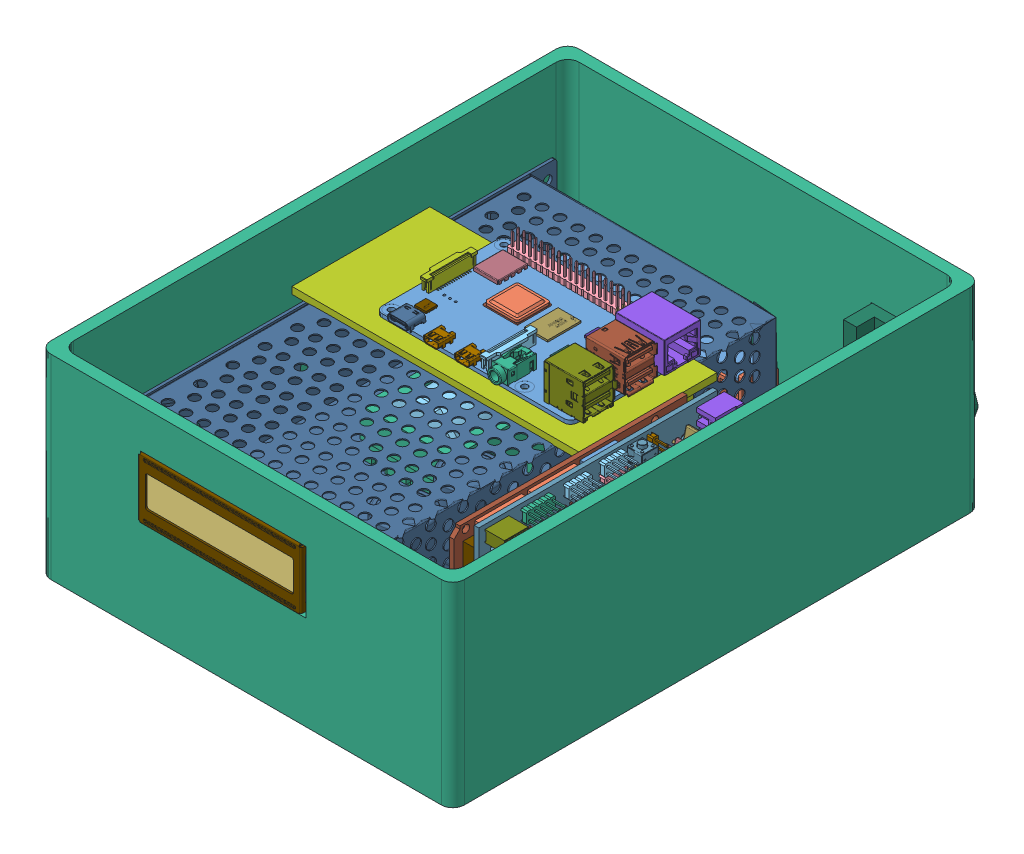
SolidWorks assembly Desktop_Arm_Assembly, configuration Default. Lengths in mm.
Overall size (180 85 238.3).
199 component instances, 97 part files, 19 mates.
Components (placement in the parent):
- Raspberry Pi 4 Model B-1: Raspberry Pi 4 Model B [Default] at (14.6782 37.9484 76.8197) size (88.99 19.9 58.4)
  - PCB, RPi4ModelB-1: PCB, RPi4ModelB [Default] at origin size (85 1.6 56)
  - Broadcom BCM2711B0 CPU, RPi4ModelB-1: Broadcom BCM2711B0 CPU, RPi4ModelB [Default] at (-13.25 0.8 -4.5) size (15 2.3 15)
  - 2.54 mm DUPONT MALE PIN HEADER, POE, 2X2, RPi4ModelB-1: 2.54 mm DUPONT MALE PIN HEADER, POE, 2X2, RPi4ModelB [Default] at (19 0.8 -18.5) size (5.08 11.3 5.08)
  - 2.54 mm DUPONT MALE PIN HEADER, IO, 2X20, RPi4ModelB-1: 2.54 mm DUPONT MALE PIN HEADER, IO, 2X20, RPi4ModelB [Default] at (-10 0.8 -24.5) size (50.8 11.3 5.08)
  - Camera Connector, RPi4ModelB-1: Camera Connector, RPi4ModelB [Default] at (4 0.8 16.5) x (0 0 -1) z (1 0 0) size (22.4 5.68 5.07)
  - Microphone Plug, RPi4ModelB-1: Microphone Plug, RPi4ModelB [Default] at (11.5 0.8 21.65) size (7.23 7.55 15)
  - Display Connector, RPi4ModelB-1: Display Connector, RPi4ModelB [Default] at (-38.5 0.8 0) x (0 0 1) z (-1 0 0) size (22.4 5.68 5.07)
  - Gigabit Ethernet Port, RPi4ModelB-1: Gigabit Ethernet Port, RPi4ModelB [Default] at (45.5 7.55 -17.75) x (0 0 -1) z (1 0 0) size (16.2 17.24 21.64)
  - Female Micro HDMI Connector, RPi4ModelB-2: Female Micro HDMI Connector, RPi4ModelB [Default] at (-3 0.8 27.3875) size (6.5 3.51 7.5)
  - Female Micro HDMI Connector, RPi4ModelB-3: Female Micro HDMI Connector, RPi4ModelB [Default] at (-16.5 0.8 27.3875) size (6.5 3.51 7.5)
  - Female USB Type C Connector, RPi4ModelB-1: Female USB Type C Connector, RPi4ModelB [Default] at (-31.3 0.8 26.5419) size (8.94 3.96 7.9)
  - 2X USB3.0 PORTS, RPi4ModelB-2: 2X USB3.0 PORTS, RPi4ModelB [Default] at (37.07 0.8 1) size (17.47 19.41 15.68)
  - 91D77 D9WHV 778K, 4 GB LPDDR4 SDRAM, RPi4ModelB-1: 91D77 D9WHV 778K, 4 GB LPDDR4 SDRAM, RPi4ModelB [Default] at (2.25 0.8 -4.5) size (10 0.8 14.5)
  - Cypress CYW43455 Wireless Module Cover, RPi4ModelB-1: Cypress CYW43455 Wireless Module Cover, RPi4ModelB [Default] at (-30.5 0.8 -14.5) size (11 1.6 13)
  - SD Card Slot, RPi4ModelB-1: SD Card Slot, RPi4ModelB [Default] at (-35.3 -0.8 0) x (0 0 -1) z (-1 0 0) size (11.95 1.45 11.4)
  - VIA VL805 PCIe USB 3.0 controller, RPi4ModelB-1: VIA VL805 PCIe USB 3.0 controller, RPi4ModelB [Default] at (17.5 0.8 4) size (8.8 0.8 8.8)
  - 2X USB2.0 PORTS, RPi4ModelB-1: 2X USB2.0 PORTS, RPi4ModelB [Default] at (37.065 0.65 19) size (17.87 19.16 15.33)
  - Broadcom BCM54213PE Gigabit Ethernet Transceiver, RPi4ModelB-1: Broadcom BCM54213PE Gigabit Ethernet Transceiver, RPi4ModelB [Default] at (16.5 0.8 -10) size (6.8 1 6.8)
  - MxL7704 Universal PMIC, RPi4ModelB-1: MxL7704 Universal PMIC, RPi4ModelB [Default] at (-32.5 0.8 16) size (5.4 0.8 5.4)
- PowerSupply_S-240-12.step-1: PowerSupply_S-240-12.step [Default] at (2.5782 -11.3016 98.3197) x (0 0 -1) z (0 1 0) size (202.29 118.05 58.32)
  - ScrewTerminalBlock_1x9.step-1: ScrewTerminalBlock_1x9.step [Default] at origin size (16 87.5 20.2)
    - SOLID007.step-1: SOLID007.step [Default] at origin size (14.65 87.4 2.8)
    - SOLID008.step-1: SOLID008.step [Default] at origin size (16 87.5 16.5)
    - SOLID009.step-1: SOLID009.step [Default] at origin size (9.8 7.4 11.5)
    - SOLID010.step-1: SOLID010.step [Default] at origin size (7.4 7.4 9.45)
    - SOLID011.step-1: SOLID011.step [Default] at origin size (9.8 7.4 11.5)
    - SOLID012.step-1: SOLID012.step [Default] at origin size (7.4 7.4 9.45)
    - SOLID013.step-1: SOLID013.step [Default] at origin size (9.8 7.4 11.5)
    - SOLID014.step-1: SOLID014.step [Default] at origin size (7.4 7.4 9.45)
    - SOLID015.step-1: SOLID015.step [Default] at origin size (9.8 7.4 11.5)
    - SOLID016.step-1: SOLID016.step [Default] at origin size (7.4 7.4 9.45)
    - SOLID017.step-1: SOLID017.step [Default] at origin size (9.8 7.4 11.5)
    - SOLID018.step-1: SOLID018.step [Default] at origin size (7.4 7.4 9.45)
    - SOLID019.step-1: SOLID019.step [Default] at origin size (9.8 7.4 11.5)
    - SOLID020.step-1: SOLID020.step [Default] at origin size (7.4 7.4 9.45)
    - SOLID021.step-1: SOLID021.step [Default] at origin size (9.8 7.4 11.5)
    - SOLID022.step-1: SOLID022.step [Default] at origin size (7.4 7.4 9.45)
    - SOLID023.step-1: SOLID023.step [Default] at origin size (9.8 7.4 11.5)
    - SOLID024.step-1: SOLID024.step [Default] at origin size (7.4 7.4 9.45)
    - SOLID025.step-1: SOLID025.step [Default] at origin size (9.8 7.4 11.5)
    - SOLID026.step-1: SOLID026.step [Default] at origin size (7.4 7.4 9.45)
  - Common_Mode_Choke.step-1: Common_Mode_Choke.step [Default] at origin size (18.5 21.5 27.15)
    - SOLID.step-1: SOLID.step [Default] at origin size (6 21.5 16.6)
    - SOLID001.step-1: SOLID001.step [Default] at origin size (18.5 16.8 21.5)
  - Trafo_TR01.step-1: Trafo_TR01.step [Default] at origin size (44 40 34.3)
    - SOLID002.step-1: SOLID002.step [Default] at origin size (31.6 28 24)
    - SOLID003.step-1: SOLID003.step [Default] at origin size (44 40 26.7)
  - Toroidal_Inductor-D30H24T030.step-1: Toroidal_Inductor-D30H24T030.step [Default] at origin size (36.95 37 26.57)
    - SOLID004.step-1: SOLID004.step [Default] at origin size (34.97 37 10)
    - SOLID005.step-1: SOLID005.step [Default] at origin size (34.97 37 10)
    - SOLID006.step-1: SOLID006.step [Default] at origin size (31.89 31.73 26.57)
  - eBom-FreeParts-1: eBom-FreeParts [Default] at origin size (202.29 118.05 58.32)
- hop dien.stp-1: hop dien.stp [Default] at (67.1652 328.6838 379.5226) x (0 -1 0) z (0 0 -1) size (61.76 43.8 111.7)
  - ARDUINO_MEGA.stp-1: ARDUINO_MEGA.stp [Default] at (319.6193 3.0542 265.0052) x (0 0 -1) z (-1 0 0) size (109.46 14.9 53.16)
    - ARDUINO_MEGA_BRD.stp-1: ARDUINO_MEGA_BRD.stp [Default] at (-33.9666 3.0673 -21.8675) x (1 0 0) z (0 1 0) size (101.46 53.16 2)
    - pin_header_aw140-eg-g02d.stp-1: pin_header_aw140-eg-g02d.stp [Default] at (16.2928 5.0673 -3.5536) x (-1 0 0) z (0 0 1) size (4.98 11.2 2.5)
    - pin_header_aw140-eg-g02d.stp-2: pin_header_aw140-eg-g02d.stp [Default] at (16.2928 5.0673 1.5635) x (-1 0 0) z (0 0 1) size (4.98 11.2 2.5)
    - pin_header_aw140-eg-g02d.stp-3: pin_header_aw140-eg-g02d.stp [Default] at (16.2928 5.0673 -1.1197) x (-1 0 0) z (0 0 1) size (4.98 11.2 2.5)
    - User Library-Arduino Mega_DC POWER JACK.stp-1: User Library-Arduino Mega_DC POWER JACK.stp [Default] at (-53.3977 5.0673 16.2059) x (0 0 1) z (-1 0 0) size (9.47 14.78 14.48)
    - User Library-Arduino Mega_USB SM host.stp-1: User Library-Arduino Mega_USB SM host.stp [Default] at (-48.1477 10.3173 -12.8661) x (0 0 1) z (-1 0 0) size (14.86 14.22 16.5)
    - User Library-Arduino Mega_Atmega1280 (WGL).stp-1: User Library-Arduino Mega_Atmega1280 (WGL).stp [Default] at (2.1792 5.0673 -1.4897) size (14 0.7 14)
    - User Library-Arduino Mega_tactile BUTTON.stp-1: User Library-Arduino Mega_tactile BUTTON.stp [Default] at (25.3856 5.0673 -0.9155) x (1 0 0) z (0 1 0) size (7.9 6.2 7.35)
    - User Library-Arduino Mega_SM LED.stp-1: User Library-Arduino Mega_SM LED.stp [Default] at (27.6088 5.0673 -9.939) size (2.8 1.12 1.4)
    - User Library-Arduino Mega_PIN HEADER FEMALE 2X18SLDPRT.stp-1: User Library-Arduino Mega_PIN HEADER FEMALE 2X18SLDPRT.stp [Default] at (47.9279 5.0673 19.0874) x (0 0 -1) z (1 0 0) size (45.04 8.3 5.08)
    - User Library-Arduino Mega_PIN HEADER FEMALE 6.stp-1: User Library-Arduino Mega_PIN HEADER FEMALE 6.stp [Default] at (-15.6783 5.0673 24.2251) size (15.24 8.3 2.54)
    - User Library-Arduino Mega_PIN HEADER FEMALE 8.stp-1: User Library-Arduino Mega_PIN HEADER FEMALE 8.stp [Default] at (2.1049 5.0673 24.3138) size (20.32 8.3 2.54)
    - User Library-Arduino Mega_PIN HEADER FEMALE 8.stp-2: User Library-Arduino Mega_PIN HEADER FEMALE 8.stp [Default] at (24.9983 5.0673 24.3138) size (20.32 8.3 2.54)
    - User Library-Arduino Mega_PIN HEADER FEMALE 8.stp-3: User Library-Arduino Mega_PIN HEADER FEMALE 8.stp [Default] at (19.9514 5.0673 -23.9148) size (20.32 8.3 2.54)
    - User Library-Arduino Mega_PIN HEADER FEMALE 8.stp-4: User Library-Arduino Mega_PIN HEADER FEMALE 8.stp [Default] at (-2.8895 5.0673 -23.9148) size (20.32 8.3 2.54)
    - User Library-Arduino Mega_PIN HEADER FEMALE 8.stp-5: User Library-Arduino Mega_PIN HEADER FEMALE 8.stp [Default] at (-24.6796 5.0673 -23.9148) size (20.32 8.3 2.54)
    - pin_header_aw254-dg-g06d.stp-1: pin_header_aw254-dg-g06d.stp [Default] at (-30.3155 5.0673 -19.3157) x (1 0 0) z (0 0 -1) size (7.62 11.5 5.08)
  - RAMPS1_4.stp-1: RAMPS1_4.stp [Default] at (314.7148 -10.7327 258.615) x (0 0 -1) z (-1 0 0) size (106.85 37.63 61.76)
    - User Library-CAPSMD6_3x3_9.stp-1: User Library-CAPSMD6_3x3_9.stp [Default] at (-23.4034 4.2803 -13.8521) x (0 0 -1) z (0 1 0) size (6.6 7 3.91)
      - User Library-CAPSMD6_3x3_9_CAP003.stp-1: User Library-CAPSMD6_3x3_9_CAP003.stp [Default] at origin size (0.65 2.6 0.32)
      - User Library-CAPSMD6_3x3_9_CAP.stp-1: User Library-CAPSMD6_3x3_9_CAP.stp [Default] at origin size (6.3 6.3 3.26)
      - User Library-CAPSMD6_3x3_9_CAP001.stp-1: User Library-CAPSMD6_3x3_9_CAP001.stp [Default] at origin size (6.6 6.6 0.64)
      - User Library-CAPSMD6_3x3_9_CAP002.stp-1: User Library-CAPSMD6_3x3_9_CAP002.stp [Default] at origin size (5.11 1.47 0.01)
      - User Library-CAPSMD6_3x3_9_CAP004.stp-1: User Library-CAPSMD6_3x3_9_CAP004.stp [Default] at origin size (0.65 2.6 0.32)
    - User Library-CAPSMD6_3x3_9.stp-2: User Library-CAPSMD6_3x3_9.stp [Default] at (-2.2688 4.2803 -13.8521) x (0 0 -1) z (0 1 0) size (6.6 7 3.91)
      - User Library-CAPSMD6_3x3_9_CAP003.stp-1: User Library-CAPSMD6_3x3_9_CAP003.stp [Default] at origin size (0.65 2.6 0.32)
      - User Library-CAPSMD6_3x3_9_CAP.stp-1: User Library-CAPSMD6_3x3_9_CAP.stp [Default] at origin size (6.3 6.3 3.26)
      - User Library-CAPSMD6_3x3_9_CAP001.stp-1: User Library-CAPSMD6_3x3_9_CAP001.stp [Default] at origin size (6.6 6.6 0.64)
      - User Library-CAPSMD6_3x3_9_CAP002.stp-1: User Library-CAPSMD6_3x3_9_CAP002.stp [Default] at origin size (5.11 1.47 0.01)
      - User Library-CAPSMD6_3x3_9_CAP004.stp-1: User Library-CAPSMD6_3x3_9_CAP004.stp [Default] at origin size (0.65 2.6 0.32)
    - User Library-CAPSMD6_3x3_9.stp-3: User Library-CAPSMD6_3x3_9.stp [Default] at (-2.8787 4.2803 9.2865) x (0 0 -1) z (0 1 0) size (6.6 7 3.91)
      - User Library-CAPSMD6_3x3_9_CAP003.stp-1: User Library-CAPSMD6_3x3_9_CAP003.stp [Default] at origin size (0.65 2.6 0.32)
      - User Library-CAPSMD6_3x3_9_CAP.stp-1: User Library-CAPSMD6_3x3_9_CAP.stp [Default] at origin size (6.3 6.3 3.26)
      - User Library-CAPSMD6_3x3_9_CAP001.stp-1: User Library-CAPSMD6_3x3_9_CAP001.stp [Default] at origin size (6.6 6.6 0.64)
      - User Library-CAPSMD6_3x3_9_CAP002.stp-1: User Library-CAPSMD6_3x3_9_CAP002.stp [Default] at origin size (5.11 1.47 0.01)
      - User Library-CAPSMD6_3x3_9_CAP004.stp-1: User Library-CAPSMD6_3x3_9_CAP004.stp [Default] at origin size (0.65 2.6 0.32)
    - User Library-CAPSMD6_3x3_9.stp-4: User Library-CAPSMD6_3x3_9.stp [Default] at (-23.2996 4.2803 9.2865) x (0 0 -1) z (0 1 0) size (6.6 7 3.91)
      - User Library-CAPSMD6_3x3_9_CAP003.stp-1: User Library-CAPSMD6_3x3_9_CAP003.stp [Default] at origin size (0.65 2.6 0.32)
      - User Library-CAPSMD6_3x3_9_CAP.stp-1: User Library-CAPSMD6_3x3_9_CAP.stp [Default] at origin size (6.3 6.3 3.26)
      - User Library-CAPSMD6_3x3_9_CAP001.stp-1: User Library-CAPSMD6_3x3_9_CAP001.stp [Default] at origin size (6.6 6.6 0.64)
      - User Library-CAPSMD6_3x3_9_CAP002.stp-1: User Library-CAPSMD6_3x3_9_CAP002.stp [Default] at origin size (5.11 1.47 0.01)
      - User Library-CAPSMD6_3x3_9_CAP004.stp-1: User Library-CAPSMD6_3x3_9_CAP004.stp [Default] at origin size (0.65 2.6 0.32)
    - User Library-CAPSMD6_3x3_9.stp-5: User Library-CAPSMD6_3x3_9.stp [Default] at (17.5196 4.2803 9.2865) x (0 0 -1) z (0 1 0) size (6.6 7 3.91)
      - User Library-CAPSMD6_3x3_9_CAP003.stp-1: User Library-CAPSMD6_3x3_9_CAP003.stp [Default] at origin size (0.65 2.6 0.32)
      - User Library-CAPSMD6_3x3_9_CAP.stp-1: User Library-CAPSMD6_3x3_9_CAP.stp [Default] at origin size (6.3 6.3 3.26)
      - User Library-CAPSMD6_3x3_9_CAP001.stp-1: User Library-CAPSMD6_3x3_9_CAP001.stp [Default] at origin size (6.6 6.6 0.64)
      - User Library-CAPSMD6_3x3_9_CAP002.stp-1: User Library-CAPSMD6_3x3_9_CAP002.stp [Default] at origin size (5.11 1.47 0.01)
      - User Library-CAPSMD6_3x3_9_CAP004.stp-1: User Library-CAPSMD6_3x3_9_CAP004.stp [Default] at origin size (0.65 2.6 0.32)
    - User Library-CAPSMD6_3x3_9.stp-6: User Library-CAPSMD6_3x3_9.stp [Default] at (-24.6073 4.2803 -1.0117) x (0 0 -1) z (0 1 0) size (6.6 7 3.91)
      - User Library-CAPSMD6_3x3_9_CAP003.stp-1: User Library-CAPSMD6_3x3_9_CAP003.stp [Default] at origin size (0.65 2.6 0.32)
      - User Library-CAPSMD6_3x3_9_CAP.stp-1: User Library-CAPSMD6_3x3_9_CAP.stp [Default] at origin size (6.3 6.3 3.26)
      - User Library-CAPSMD6_3x3_9_CAP001.stp-1: User Library-CAPSMD6_3x3_9_CAP001.stp [Default] at origin size (6.6 6.6 0.64)
      - User Library-CAPSMD6_3x3_9_CAP002.stp-1: User Library-CAPSMD6_3x3_9_CAP002.stp [Default] at origin size (5.11 1.47 0.01)
      - User Library-CAPSMD6_3x3_9_CAP004.stp-1: User Library-CAPSMD6_3x3_9_CAP004.stp [Default] at origin size (0.65 2.6 0.32)
    - User Library-CAPSMD4x3_9.stp-1: User Library-CAPSMD4x3_9.stp [Default] at (22.2937 4.2803 -15.1178) x (1 0 0) z (0 1 0) size (4.3 4.6 3.91)
      - User Library-CAPSMD4x3_9_CAPSMD4x3_9003.stp-1: User Library-CAPSMD4x3_9_CAPSMD4x3_9003.stp [Default] at origin size (0.65 1.8 0.32)
      - User Library-CAPSMD4x3_9_CAPSMD4x3_9004.stp-1: User Library-CAPSMD4x3_9_CAPSMD4x3_9004.stp [Default] at origin size (0.65 1.8 0.32)
      - User Library-CAPSMD4x3_9_CAPSMD4x3_9002.stp-1: User Library-CAPSMD4x3_9_CAPSMD4x3_9002.stp [Default] at origin size (3.12 0.9 0.01)
      - User Library-CAPSMD4x3_9_CAPSMD4x3_9001.stp-1: User Library-CAPSMD4x3_9_CAPSMD4x3_9001.stp [Default] at origin size (4 4 3.26)
      - User Library-CAPSMD4x3_9_CAPSMD4x3_9.stp-1: User Library-CAPSMD4x3_9_CAPSMD4x3_9.stp [Default] at origin size (4.3 4.3 0.64)
    - User Library-CAPSMD4x3_9.stp-2: User Library-CAPSMD4x3_9.stp [Default] at (27.5508 4.2803 -15.1178) x (1 0 0) z (0 1 0) size (4.3 4.6 3.91)
      - User Library-CAPSMD4x3_9_CAPSMD4x3_9003.stp-1: User Library-CAPSMD4x3_9_CAPSMD4x3_9003.stp [Default] at origin size (0.65 1.8 0.32)
      - User Library-CAPSMD4x3_9_CAPSMD4x3_9004.stp-1: User Library-CAPSMD4x3_9_CAPSMD4x3_9004.stp [Default] at origin size (0.65 1.8 0.32)
      - User Library-CAPSMD4x3_9_CAPSMD4x3_9002.stp-1: User Library-CAPSMD4x3_9_CAPSMD4x3_9002.stp [Default] at origin size (3.12 0.9 0.01)
      - User Library-CAPSMD4x3_9_CAPSMD4x3_9001.stp-1: User Library-CAPSMD4x3_9_CAPSMD4x3_9001.stp [Default] at origin size (4 4 3.26)
      - User Library-CAPSMD4x3_9_CAPSMD4x3_9.stp-1: User Library-CAPSMD4x3_9_CAPSMD4x3_9.stp [Default] at origin size (4.3 4.3 0.64)
    - User Library-CAPSMD4x3_9.stp-3: User Library-CAPSMD4x3_9.stp [Default] at (32.6212 4.2803 -15.1178) x (1 0 0) z (0 1 0) size (4.3 4.6 3.91)
      - User Library-CAPSMD4x3_9_CAPSMD4x3_9003.stp-1: User Library-CAPSMD4x3_9_CAPSMD4x3_9003.stp [Default] at origin size (0.65 1.8 0.32)
      - User Library-CAPSMD4x3_9_CAPSMD4x3_9004.stp-1: User Library-CAPSMD4x3_9_CAPSMD4x3_9004.stp [Default] at origin size (0.65 1.8 0.32)
      - User Library-CAPSMD4x3_9_CAPSMD4x3_9002.stp-1: User Library-CAPSMD4x3_9_CAPSMD4x3_9002.stp [Default] at origin size (3.12 0.9 0.01)
      - User Library-CAPSMD4x3_9_CAPSMD4x3_9001.stp-1: User Library-CAPSMD4x3_9_CAPSMD4x3_9001.stp [Default] at origin size (4 4 3.26)
      - User Library-CAPSMD4x3_9_CAPSMD4x3_9.stp-1: User Library-CAPSMD4x3_9_CAPSMD4x3_9.stp [Default] at origin size (4.3 4.3 0.64)
    - RAMPS1_4_1.stp-1: RAMPS1_4_1.stp [Default] at (-38.4421 2.2803 -26.502) x (1 0 0) z (0 1 0) size (103.85 61.76 2)
    - User Library-POWER MOSFET, NON-SURFACE-MOUNT.stp-1: User Library-POWER MOSFET, NON-SURFACE-MOUNT.stp [Default] at (-31.1839 8.1208 -13.4695) x (-1 0 0) z (0 -1 0) size (9.65 4.5 28.38)
    - female_header_a-bl254-dg-g08d.stp-1: female_header_a-bl254-dg-g08d.stp [Default] at (41.0483 4.2583 25.6311) size (10.41 11.65 5)
    - female_header_a-bl254-eg-g08d.stp-1: female_header_a-bl254-eg-g08d.stp [Default] at (6.4047 4.2963 4.0858) size (20.57 11.65 2.5)
    - female_header_a-bl254-eg-g08d.stp-2: female_header_a-bl254-eg-g08d.stp [Default] at (6.3863 4.2963 -6.1397) size (20.57 11.65 2.5)
    - female_header_a-bl254-eg-g08d.stp-3: female_header_a-bl254-eg-g08d.stp [Default] at (-14.6923 4.2963 -6.1397) size (20.57 11.65 2.5)
    - female_header_a-bl254-eg-g08d.stp-4: female_header_a-bl254-eg-g08d.stp [Default] at (-14.6047 4.2963 -18.9127) size (20.57 11.65 2.5)
    - female_header_a-bl254-eg-g08d.stp-5: female_header_a-bl254-eg-g08d.stp [Default] at (6.3793 4.2963 -18.9127) size (20.57 11.65 2.5)
    - female_header_a-bl254-eg-g08d.stp-6: female_header_a-bl254-eg-g08d.stp [Default] at (6.414 4.2963 16.9123) size (20.57 11.65 2.5)
    - female_header_a-bl254-eg-g08d.stp-7: female_header_a-bl254-eg-g08d.stp [Default] at (-13.9941 4.2963 16.9123) size (20.57 11.65 2.5)
    - female_header_a-bl254-eg-g08d.stp-8: female_header_a-bl254-eg-g08d.stp [Default] at (-14.0103 4.2963 4.0799) size (20.57 11.65 2.5)
    - female_header_a-bl254-eg-g08d.stp-9: female_header_a-bl254-eg-g08d.stp [Default] at (26.8453 4.2963 4.0799) size (20.57 11.65 2.5)
    - female_header_a-bl254-eg-g08d.stp-10: female_header_a-bl254-eg-g08d.stp [Default] at (26.8273 4.2963 16.9325) size (20.57 11.65 2.5)
    - pin_header_aw254-dg-g36d.stp-1: pin_header_aw254-dg-g36d.stp [Default] at (40.9113 2.2243 -7.3898) x (0 0 1) z (-1 0 0) size (45.72 11.5 5.08)
    - pin_header_aw140-eg-g18d.stp-1: pin_header_aw140-eg-g18d.stp [Default] at (44.7503 4.3173 -7.3949) x (0 0 -1) z (-1 0 0) size (45.62 11.2 2.5)
    - pin_header_aw140-eg-g08d.stp-1: pin_header_aw140-eg-g08d.stp [Default] at (28.1033 2.2803 19.4616) size (20.22 11.2 2.5)
    - pin_header_aw140-eg-g08d.stp-2: pin_header_aw140-eg-g08d.stp [Default] at (5.0609 2.2803 19.4616) size (20.22 11.2 2.5)
    - pin_header_aw140-eg-g08d.stp-3: pin_header_aw140-eg-g08d.stp [Default] at (-0.0426 2.2803 -29.0108) size (20.22 11.2 2.5)
    - pin_header_aw140-eg-g08d.stp-4: pin_header_aw140-eg-g08d.stp [Default] at (22.8713 2.2803 -29.0108) size (20.22 11.2 2.5)
    - pin_header_aw140-eg-g08d.stp-5: pin_header_aw140-eg-g08d.stp [Default] at (-21.773 2.2803 -29.0108) size (20.22 11.2 2.5)
    - pin_header_aw140-eg-g06d.stp-1: pin_header_aw140-eg-g06d.stp [Default] at (29.4382 4.2803 -6.1813) x (-1 0 0) z (0 0 1) size (15.14 11.2 2.5)
    - pin_header_aw140-eg-g06d.stp-2: pin_header_aw140-eg-g06d.stp [Default] at (26.2798 4.2623 -19.3796) x (-1 0 0) z (0 0 1) size (15.14 11.2 2.5)
    - pin_header_aw140-eg-g06d.stp-3: pin_header_aw140-eg-g06d.stp [Default] at (26.2798 4.2623 -21.9464) x (-1 0 0) z (0 0 1) size (15.14 11.2 2.5)
    - pin_header_aw140-eg-g06d.stp-4: pin_header_aw140-eg-g06d.stp [Default] at (26.2798 4.2623 -24.4908) x (-1 0 0) z (0 0 1) size (15.14 11.2 2.5)
    - pin_header_aw140-eg-g04d.stp-1: pin_header_aw140-eg-g04d.stp [Default] at (8.4073 4.2803 -24.0519) x (-1 0 0) z (0 0 1) size (10.06 11.2 2.5)
    - pin_header_aw140-eg-g04d.stp-2: pin_header_aw140-eg-g04d.stp [Default] at (-12.021 4.2623 -24.0519) x (-1 0 0) z (0 0 1) size (10.06 11.2 2.5)
    - pin_header_aw140-eg-g04d.stp-3: pin_header_aw140-eg-g04d.stp [Default] at (-8.9039 4.2623 -1.0355) x (-1 0 0) z (0 0 1) size (10.06 11.2 2.5)
    - pin_header_aw140-eg-g04d.stp-4: pin_header_aw140-eg-g04d.stp [Default] at (9.0685 4.2623 -1.0355) x (-1 0 0) z (0 0 1) size (10.06 11.2 2.5)
    - pin_header_aw140-eg-g04d.stp-5: pin_header_aw140-eg-g04d.stp [Default] at (-8.3709 4.2803 22.5944) x (-1 0 0) z (0 0 1) size (10.06 11.2 2.5)
    - pin_header_aw254-dg-g06d.stp-1: pin_header_aw254-dg-g06d.stp [Default] at (-10.2573 4.2803 9.2323) x (-1 0 0) z (0 0 1) size (7.62 11.5 5.08)
    - pin_header_aw254-dg-g06d.stp-2: pin_header_aw254-dg-g06d.stp [Default] at (10.1683 4.2623 9.2323) x (-1 0 0) z (0 0 1) size (7.62 11.5 5.08)
    - pin_header_aw254-dg-g06d.stp-3: pin_header_aw254-dg-g06d.stp [Default] at (30.6527 4.2623 9.2323) x (-1 0 0) z (0 0 1) size (7.62 11.5 5.08)
    - pin_header_aw254-dg-g06d.stp-4: pin_header_aw254-dg-g06d.stp [Default] at (10.1683 4.2623 -13.7827) x (-1 0 0) z (0 0 1) size (7.62 11.5 5.08)
    - pin_header_aw254-dg-g06d.stp-5: pin_header_aw254-dg-g06d.stp [Default] at (-10.2204 4.2623 -13.7827) x (-1 0 0) z (0 0 1) size (7.62 11.5 5.08)
    - pin_header_aw254-dg-g08d.stp-1: pin_header_aw254-dg-g08d.stp [Default] at (7.0775 4.2803 25.6017) x (-1 0 0) z (0 0 1) size (10.16 11.5 5.08)
    - pin_header_aw254-dg-g08d.stp-2: pin_header_aw254-dg-g08d.stp [Default] at (-8.3884 4.2803 26.4286) x (-1 0 0) z (0 0 1) size (10.16 11.5 5.08)
    - pin_header_aw254-dg-g10d.stp-1: pin_header_aw254-dg-g10d.stp [Default] at (24.3252 4.2803 25.6162) x (-1 0 0) z (0 0 1) size (12.7 11.5 5.08)
    - pin_header_aw140-eg-g04d.stp-6: pin_header_aw140-eg-g04d.stp [Default] at (35.1498 4.2623 -23.186) x (0 0 -1) z (-1 0 0) size (10.06 11.2 2.5)
    - pin_header_aw140-eg-g06d.stp-5: pin_header_aw140-eg-g06d.stp [Default] at (-15.2568 2.2803 19.3514) size (15.14 11.2 2.5)
    - terminal_blocks_a-tb500-to06.stp-1: terminal_blocks_a-tb500-to06.stp [Default] at (-37.5276 4.2805 -9.866) x (0 0 1) z (-1 0 0) size (30.6 13.8 8.3)
    - terminal_blocks_a-tb508-oq04ch.stp-1: terminal_blocks_a-tb508-oq04ch.stp [Default] at (-57.9426 4.2803 17.0267) x (0 0 1) z (-1 0 0) size (22.32 12.5 12)
    - pin_header_aw254-dg-g08d.stp-3: pin_header_aw254-dg-g08d.stp [Default] at (26.8817 4.262 0.2918) x (-1 0 0) z (0 0 1) size (10.16 11.5 5.08)
    - pin_header_aw140-eg-g02d.stp-1: pin_header_aw140-eg-g02d.stp [Default] at (-26.0896 4.2803 12.3888) x (0 0 1) z (1 0 0) size (4.98 11.2 2.5)
    - pin_header_aw140-eg-g03d.stp-1: pin_header_aw140-eg-g03d.stp [Default] at (-25.5036 4.2803 24.8649) x (0 0 1) z (1 0 0) size (7.52 11.2 2.5)
    - User Library-APA3010GCCK_GREEN.stp-1: User Library-APA3010GCCK_GREEN.stp [Default] at (-34.2243 4.3303 -27.7242) x (0 0 1) z (-1 0 0) size (3 2 0.99)
    - User Library-APA3010GCCK_RED.stp-1: User Library-APA3010GCCK_RED.stp [Default] at (-49.6186 4.3303 -27.7242) x (0 0 1) z (-1 0 0) size (3 2 0.99)
    - User Library-APA3010GCCK_RED.stp-2: User Library-APA3010GCCK_RED.stp [Default] at (-52.1606 4.3303 -27.7242) x (0 0 1) z (-1 0 0) size (3 2 0.99)
    - User Library-MF-R1100___ _________.stp-1: User Library-MF-R1100___ _________.stp [Default] at (-35.8426 -0.3427 15.082) x (0 0 -1) z (0 -1 0) size (23.64 7.06 35.7)
    - User Library-MF-R500___ _________.stp-1: User Library-MF-R500___ _________.stp [Default] at (-32.3357 -0.5897 15.5605) x (0.000533 0 -1) z (0 -1 0) size (17.04 5.43 29.1)
    - User Library-SWITCH, TACTILE, RIGHT ANGLE, 12VDC, 50MA, 6_85MM ACTUATOR, WEALTH METAL TC-0244Z.stp-1: User Library-SWITCH, TACTILE, RIGHT ANGLE, 12VDC, 50MA, 6_85MM ACTUATOR, WEALTH METAL TC-0244Z.stp [Default] at (-19.0613 3.9803 23.5512) size (7.4 11 8)
    - User Library-APA3010GCCK_RED.stp-3: User Library-APA3010GCCK_RED.stp [Default] at (-29.5185 4.3303 -5.1301) size (3 2 0.99)
    - User Library-POWER MOSFET, NON-SURFACE-MOUNT.stp-2: User Library-POWER MOSFET, NON-SURFACE-MOUNT.stp [Default] at (-31.3941 8.4328 -20.0341) x (-1 0 0) z (0 -1 0) size (9.65 4.5 28.38)
    - User Library-POWER MOSFET, NON-SURFACE-MOUNT.stp-3: User Library-POWER MOSFET, NON-SURFACE-MOUNT.stp [Default] at (-36.1067 8.2818 -5.2135) x (0 0 -1) z (0 -1 0) size (9.65 4.5 28.38)
- AC Input Connector and Switch.step-1: AC Input Connector and Switch.step [Default] at (87.9782 11.6984 -13.8803) x (1 0 0) z (0 0 -1) size (49.46 54 40.3)
- LCD.STEP-1: LCD.STEP [Default] at (15.6782 33.1984 206.4197) x (1 0 0) z (0 -1 0) size (80 18.3 36)
  - pcbboard.STEP-1: pcbboard.STEP [Default] at origin size (80 4.19 36)
  - 16pin_header__.STEP-1: 16pin_header__.STEP [Default] at (-32 0 -15.5) x (0 0 1) z (1 0 0) size (2.54 11.5 40.64)
  - lcd window.STEP-1: lcd window.STEP [Default] at (0 9 1.5) size (71.3 11.8 27.44)
  - backlight.STEP-1: backlight.STEP [Default] at (0 1.7 1.5) x (-1 0 0) z (0 0 -1) size (74.38 2.98 18)
  - conductor.STEP-1: conductor.STEP [Default] at (0 1.7 12.6) size (69.7 5.5 3)
  - conductor.STEP-2: conductor.STEP [Default] at (0 1.7 -9.6) size (69.7 5.5 3)
  - liquid crystal grabcad.STEP-1: liquid crystal grabcad.STEP [Default] at (0 7.9 1.5) size (68.5 2.2 25)
  - smt_resistor222.STEP-1: smt_resistor222.STEP [Default] at (-32.75 0 -5.25) x (0 0 1) z (1 0 0) size (1.8 0.6 4)
  - smt_resistor222.STEP-2: smt_resistor222.STEP [Default] at (-32.75 0 -2.75) x (0 0 1) z (1 0 0) size (1.8 0.6 4)
  - smt_resistor222.STEP-3: smt_resistor222.STEP [Default] at (-32.75 0 -0.25) x (0 0 1) z (1 0 0) size (1.8 0.6 4)
  - smt_resistor222.STEP-4: smt_resistor222.STEP [Default] at (-32.75 0 2.25) x (0 0 1) z (1 0 0) size (1.8 0.6 4)
  - smt_resistor222.STEP-5: smt_resistor222.STEP [Default] at (-32.75 0 4.75) x (0 0 1) z (1 0 0) size (1.8 0.6 4)
  - smt_resistor222.STEP-6: smt_resistor222.STEP [Default] at (-32.75 0 7.25) x (0 0 1) z (1 0 0) size (1.8 0.6 4)
  - smt_resistor101.STEP-1: smt_resistor101.STEP [Default] at (30.25 0 6.1) x (0 0 -1) z (-1 0 0) size (1.8 0.6 5.2)
  - smt_resistor101.STEP-2: smt_resistor101.STEP [Default] at (30.25 0 2.85) x (0 0 -1) z (-1 0 0) size (1.8 0.6 5.2)
- Bottom-1: Bottom [Default] at (117.1782 -22.3016 216.1197) x (0 0 -1) z (1 0 0) size (230 85 180)
- Raspi Shelf-1: Raspi Shelf [Default] at (67.1782 32.6984 51.1197) x (-1 0 0) z (0 0 -1) size (125 53 60)
Mates (geometry in assembly coordinates):
- Coincident1: coincident anti-aligned: plane of AC Input Connector and Switch.step-1 through (117.9782 11.6984 -13.8803) normal (0 0 1); plane of Bottom-1 through (147.1782 -17.3016 -13.8803) normal (0 0 -1)
- Concentric1: concentric aligned: circle of AC Input Connector and Switch.step-1; cylinder of Bottom-1 through (138.1782 11.6984 -8.8803) axis (0 0 -1) radius 1.5
- Concentric3: concentric aligned: circle of AC Input Connector and Switch.step-1; circle of Bottom-1
- Coincident4: coincident anti-aligned: plane of PowerSupply_S-240-12.step-1/eBom-FreeParts-1 through (-22.8218 -17.3016 201.1197) normal (0 -1 0); plane of Bottom-1 through (147.1782 -17.3016 216.1197) normal (0 1 0)
- Distance1: distance = 5 mm anti-aligned: plane of PowerSupply_S-240-12.step-1/eBom-FreeParts-1 through (-52.8218 32.6984 201.1197) normal (-1 0 0); plane of Bottom-1 through (-57.8218 62.6984 211.1197) normal (1 0 0)
- Distance2: distance = 10 mm anti-aligned: plane of PowerSupply_S-240-12.step-1/eBom-FreeParts-1 through (-14.3892 -8.869 201.1197) normal (0 0 1); plane of Bottom-1 through (112.1782 62.6984 211.1197) normal (0 0 -1)
- Concentric7: concentric aligned: circle of LCD.STEP-1/pcbboard.STEP-1; circle of Bottom-1
- Concentric8: concentric aligned: circle of LCD.STEP-1/pcbboard.STEP-1; circle of Bottom-1
- Coincident12: coincident anti-aligned: plane of LCD.STEP-1/pcbboard.STEP-1 through (45.6782 33.1984 208.1197) normal (0 0 1); plane of Bottom-1 through (8.1782 48.6984 208.1197) normal (0 0 -1)
- Coincident13: coincident anti-aligned: plane of hop dien.stp-1/ARDUINO_MEGA.stp-1/ARDUINO_MEGA_BRD.stp-1 through (89.1782 -17.3016 66.1197) normal (0 -1 0); plane of Bottom-1 through (147.1782 -17.3016 216.1197) normal (0 1 0)
- Distance3: distance = 125 mm anti-aligned: plane of hop dien.stp-1/ARDUINO_MEGA.stp-1/ARDUINO_MEGA_BRD.stp-1 through (67.1782 -12.803 80.5508) normal (-1 0 0); plane of Bottom-1 through (-57.8218 62.6984 211.1197) normal (1 0 0)
- Distance4: distance = 70 mm anti-aligned: plane of Bottom-1 through (112.1782 62.6984 -8.8803) normal (0 0 1); plane of hop dien.stp-1/ARDUINO_MEGA.stp-1/User Library-Arduino Mega_DC POWER JACK.stp-1 through (80.3542 20.6984 61.1197) normal (0 0 -1)
- Coincident16: coincident anti-aligned: plane of Bottom-1 through (147.1782 -17.3016 216.1197) normal (0 1 0); plane of Raspi Shelf-1 through (92.1782 -17.3016 101.1197) normal (0 -1 0)
- Coincident17: coincident anti-aligned: plane of Bottom-1 through (-27.8218 62.6984 211.1197) normal (1 0 0); plane of Raspi Shelf-1 through (-27.8218 35.6984 51.1197) normal (-1 0 0)
- Distance5: distance = 60 mm anti-aligned: plane of Bottom-1 through (112.1782 62.6984 -8.8803) normal (0 0 1); plane of Raspi Shelf-1 through (67.1782 35.6984 51.1197) normal (0 0 -1)
- Parallel4: parallel anti-aligned: plane of Raspberry Pi 4 Model B-1/PCB, RPi4ModelB-1 through (-27.8218 38.7484 48.8197) normal (-1 0 0); plane of Bottom-1 through (-27.8218 62.6984 211.1197) normal (1 0 0)
- Distance6: distance = 0 mm aligned: plane of Raspberry Pi 4 Model B-1/Gigabit Ethernet Port, RPi4ModelB-1 through (60.1782 38.7484 51.1197) normal (0 0 -1); plane of Raspi Shelf-1 through (67.1782 35.6984 51.1197) normal (0 0 -1)
- Distance8: distance = 30 mm anti-aligned: plane of Raspberry Pi 4 Model B-1/PCB, RPi4ModelB-1 through (-27.8218 38.7484 48.8197) normal (-1 0 0); plane of Bottom-1 through (-57.8218 62.6984 211.1197) normal (1 0 0)
- Coincident27: coincident anti-aligned: plane of Raspberry Pi 4 Model B-1/SD Card Slot, RPi4ModelB-1 through (-14.9208 35.6984 82.5007) normal (0 -1 0); plane of Raspi Shelf-1 through (97.1782 35.6984 51.1197) normal (0 1 0)
